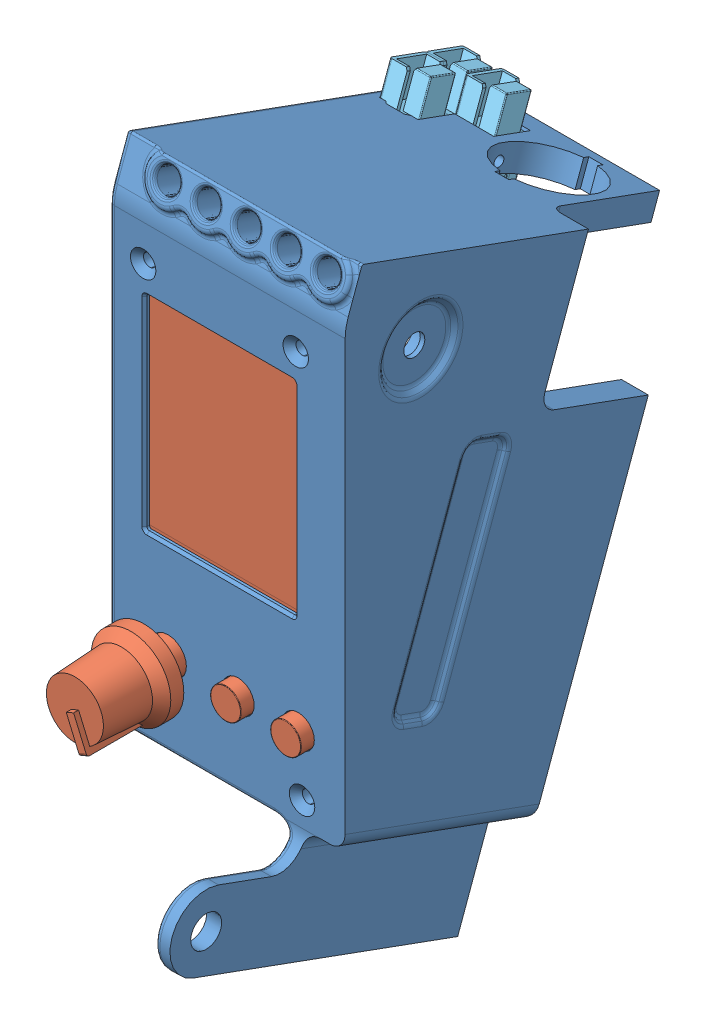
SolidWorks assembly AxxSolder_JBC-AD-SF, configuration Default. Lengths in mm.
Overall size (47.1 134.17 107.8).
8 component instances, 5 part files, 9 mates.
Components (placement in the parent):
- Encolsure_JBC-AD-SF-1: Encolsure_JBC-AD-SF [Default] at (87.8631 11.8541 -194.6908) x (0 -0.939693 0.34202) z (-1 0 0) size (116.45 72.33 47.1)
- AxxSolder-1: AxxSolder [Default] at (82.2631 -57.9029 -136.8216) size (39.06 82.5 39.41)
- Mounting_Bracket_A-1: Mounting_Bracket_A [Default] at (62.7631 -54.9029 -140.8216) x (1 0 0) z (0 1 0) size (37.5 7 4.5)
- Mounting_Bracket_B-1: Mounting_Bracket_B [Default] at (62.7831 22.0991 -140.8216) x (1 0 0) z (0 1 0) size (34.98 7 4.5)
- Anderson_PowerPole-1: Anderson_PowerPole [Default] at (46.9346 2.4207 -184.2187) x (0 -0.34202 -0.939693) z (0 0.939693 -0.34202) size (16.24 16.24 22.71)
  - powerpole 15-45A housing.step-3: powerpole 15-45A housing.step [Default] at origin size (8.44 8.44 22.71)
  - powerpole 15-45A housing.step-5: powerpole 15-45A housing.step [Default] at (-7.8 0 0) size (8.44 8.44 22.71)
  - powerpole 15-45A housing.step-6: powerpole 15-45A housing.step [Default] at (0 -7.8 0) size (8.44 8.44 22.71)
Mates (geometry in assembly coordinates):
- Coincident1: coincident anti-aligned: plane of Encolsure_JBC-AD-SF-1 through (43.0131 11.8541 -194.6908) normal (1 0 0); plane of Anderson_PowerPole-1/powerpole 15-45A housing.step-5 through (43.0131 28.6376 -181.3251) normal (-1 0 0)
- Coincident3: coincident anti-aligned: plane of Encolsure_JBC-AD-SF-1 through (43.0131 14.6569 -192.8377) normal (0 0.34202 0.939693); plane of Anderson_PowerPole-1/powerpole 15-45A housing.step-6 through (50.8131 23.3021 -195.9843) normal (0 -0.34202 -0.939693)
- Distance2: distance = 6.2 mm aligned: plane of Anderson_PowerPole-1/powerpole 15-45A housing.step-3 through (50.8131 25.9698 -188.6547) normal (0 0.939693 -0.34202); plane of Encolsure_JBC-AD-SF-1 through (-3.5201 16.5525 -196.4009) normal (0 0.939693 -0.34202)
- Concentric1: concentric aligned: cylinder of Encolsure_JBC-AD-SF-1 through (46.2631 -54.9029 -137.5916) axis (0 0 1) radius 1.25; cylinder of AxxSolder-1 through (46.2631 -54.9029 -136.8316) axis (0 0 1) radius 1.25
- Coincident4: coincident anti-aligned: plane of Encolsure_JBC-AD-SF-1 through (44.0131 -51.8529 -135.2216) normal (0 0 -1); plane of AxxSolder-1 through (62.7631 -16.6529 -135.2216) normal (0 0 1)
- Coincident5: coincident anti-aligned: plane of AxxSolder-1 through (62.7631 -16.6529 -136.8216) normal (0 0 -1); plane of Mounting_Bracket_A-1 through (62.7631 -54.9029 -136.8216) normal (0 0 1)
- Concentric3: concentric aligned: cylinder of AxxSolder-1 through (46.2631 -54.9029 -136.8316) axis (0 0 1) radius 1.25; cylinder of Mounting_Bracket_A-1 through (46.2631 -54.9029 -143.8216) axis (0 0 1) radius 1
- Concentric4: concentric aligned: cylinder of AxxSolder-1 through (47.5431 22.0991 -136.8316) axis (0 0 1) radius 1.25; cylinder of Mounting_Bracket_B-1 through (47.5431 22.0991 -143.8216) axis (0 0 1) radius 1
- Coincident6: coincident anti-aligned: plane of AxxSolder-1 through (62.7631 -16.6529 -136.8216) normal (0 0 -1); plane of Mounting_Bracket_B-1 through (62.7831 22.0991 -136.8216) normal (0 0 1)
